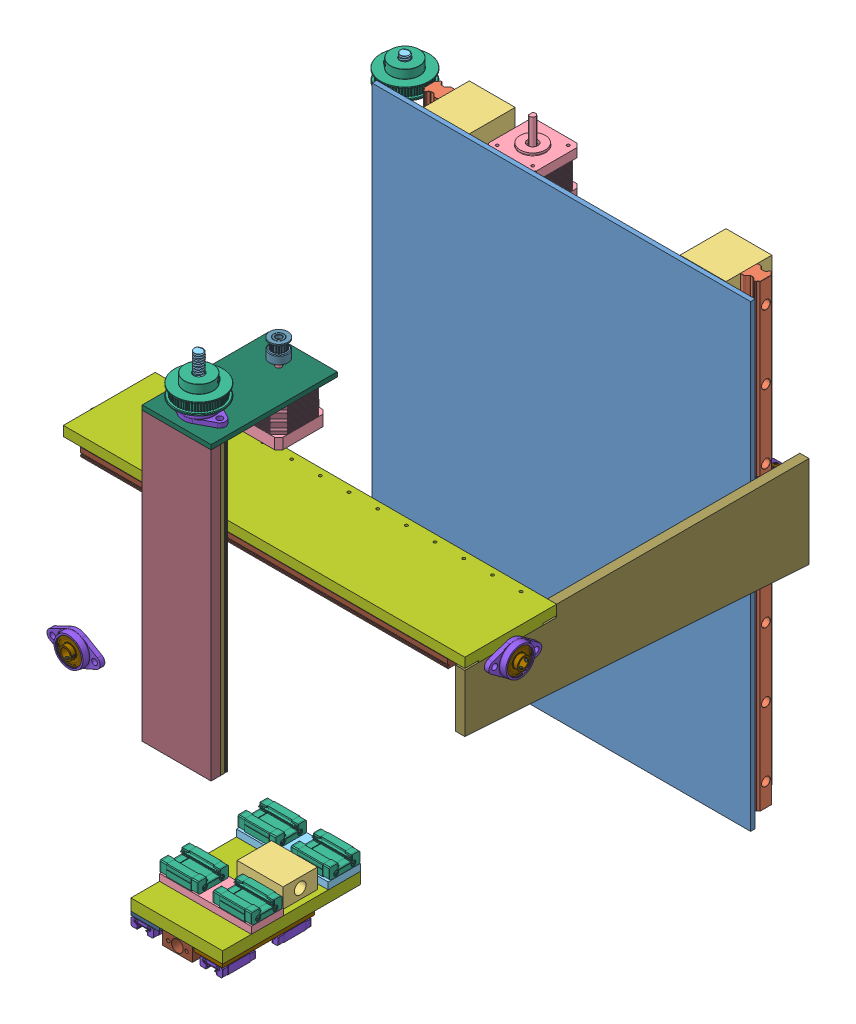
SolidWorks assembly Fresa_190421_2259, configuration Predeterminado. Lengths in mm.
Overall size (378.35 507.31 471.29).
73 component instances, 35 part files, 0 mates.
Components (placement in the parent):
- Mesa^Fresa_190421_2259-1: Mesa^Fresa_190421_2259 [Predeterminado] at (-186.1122 103.6393 -218.5133) x (0 -1 0) z (0 0 1) size (400 330 4) (virtual)
- HGR15R Rail-1: HGR15R Rail [HGR15R400CE20] at (-145.2122 -296.3607 -238.5133) x (0 0 1) z (0 -1 0) size (15 15 400)
- perfil_4040^Fresa_190421_2259-1: perfil_4040^Fresa_190421_2259 [Predeterminado] at (-145.3622 103.6393 -258.5133) x (1 0 0) z (0 -1 0) size (40 40 400) (virtual)
- HGR15R Rail-2: HGR15R Rail [HGR15R400CE20] at (117.8878 -296.3607 -238.8633) x (0 0 -1) z (0 -1 0) size (15 15 400)
- perfil_4040^Fresa_190421_2259-2: perfil_4040^Fresa_190421_2259 [Predeterminado] at (78.0378 103.6393 -258.8633) x (1 0 0) z (0 -1 0) size (40 40 400) (virtual)
- Nema 17HS4401-S-2: Nema 17HS4401-S [Varsayılan] at (-71.0952 61.4393 -239.5133) x (0 0 -1) z (0 1 0) size (42 48 63.23)
- LeadScrew 8mm x 2mmPitch-2: LeadScrew 8mm x 2mmPitch [Default] at (-180.6122 117.9173 -237.6496) x (0.520198 0 -0.854046) z (0 1 0) size (9.24 8 301.1)
- GT2_60T_8_6-2: GT2_60T_8_6 [Default] at (-180.6122 106.533 -237.6496) x (-0.750477 0 -0.660897) z (0 -1 0) size (42 42 18)
- Eje_X^Fresa_190421_2259-1: Eje_X^Fresa_190421_2259 [Predeterminado] at (0 -20.7118 0) size (378.35 85.52 428.57) (virtual)
  - Copia de Placa_X^Eje_X_Fresa_190421_2259-1: Copia de Placa_X^Eje_X_Fresa_190421_2259 [Predeterminado] at (-196.1122 -9.5232 -35.4133) x (1 0 0) z (0 -1 0) size (350 80 10) (virtual)
  - KFL08-1: KFL08 [Varsayılan] at (-66.4126 -53.0232 161.3598) x (0.999067 -0.043192 0) z (-0.043192 -0.999067 0) size (46.5 11.35 27)
    - FLANGE^KFL08-1: FLANGE^KFL08 [Default] at origin size (46.5 8.5 27) (virtual)
    - BEARING^KFL08-1: BEARING^KFL08 [Default] at (0 4 0) x (1 0 0) z (0 -1 0) size (22 22 10.85) (virtual)
    - socket set screw cone point_am-1: socket set screw cone point_am [B18.3.6M - M2.5 x 0.45 x 2 Hex Socket Cone Pt. SS --S] at (0 9.425 5.45) x (0 0 -1) z (1 0 0) size (2 2.5 2.5)
    - socket set screw cone point_am-2: socket set screw cone point_am [B18.3.6M - M2.5 x 0.45 x 2 Hex Socket Cone Pt. SS --S] at (5.45 9.425 0) x (-1 0 0) z (0 0 -1) size (2 2.5 2.5)
  - LeadScrew 8mm x 2mmPitch-1: LeadScrew 8mm x 2mmPitch [Default] at (-212.2662 -28.5232 4.5867) x (0 0.930056 0.367419) z (-1 0 0) size (9.24 8 301.1)
  - MGN12R-320-1: MGN12R-320 [Predeterminado] at (-111.1122 -21.9725 -29.4133) x (0 0 1) z (1 0 0) size (12 8.1 320)
  - MGN12R-320-2: MGN12R-320 [Predeterminado] at (-111.1122 -21.9725 38.5867) x (0 0 1) z (1 0 0) size (12 8.1 320)
  - Copia de Columa_1^Eje_X_Fresa_190421_2259-1: Copia de Columa_1^Eje_X_Fresa_190421_2259 [Predeterminado] at (-188.1122 -29.0154 -199.7436) x (0 -1 0) z (-1 0 0) size (80 300 8) (hidden, virtual)
  - Copia de Columa_1^Eje_X_Fresa_190421_2259-2: Copia de Columa_1^Eje_X_Fresa_190421_2259 [Predeterminado] at (153.8878 -29.0154 -199.7436) x (0 -1 0) z (-1 0 0) size (80 300 8) (virtual)
  - HGH15CA-1: HGH15CA [Default] at (117.8878 -53.7232 -238.8633) x (0 0 -1) z (0 -1 0) size (34 23.7 61.49)
    - HGH15CA Block-1: HGH15CA Block [HGR15R300CE20] at origin size (34 23.7 39.4)
    - HGx15CA Retainer-1: HGx15CA Retainer [HGR15R300CE20] at origin size (26 4 55.4)
    - HGx15CA Tiny Red-1: HGx15CA Tiny Red [HGR15R300CE20] at origin size (14.2 1 55.4)
    - HGx15CA End Cap-1: HGx15CA End Cap [HGR15R300CE20] at origin size (32.5 19.5 8)
    - HGx15CA End Cap-2: HGx15CA End Cap [HGR15R300CE20] x (-1 0 0) z (0 0 -1) size (32.5 19.5 8)
    - HGx15CA Seal-1: HGx15CA Seal [HGR15R300CE20] at origin size (32.5 19.5 3)
    - HGx15CA Seal-2: HGx15CA Seal [HGR15R300CE20] x (-1 0 0) z (0 0 -1) size (32.5 19.5 3)
    - pan head cross recess screw_iso2-1: pan head cross recess screw_iso2 [ISO 7045 - M2.5 x 16 - Z - 16C] at (11.5 11.8 30.8) x (0 0 -1) z (0 -1 0) size (18.05 5 5)
    - pan head cross recess screw_iso2-2: pan head cross recess screw_iso2 [ISO 7045 - M2.5 x 16 - Z - 16C] at (-11.5 11.8 30.8) x (0 0 -1) z (0 1 0) size (18.05 5 5)
    - pan head cross recess screw_iso2-3: pan head cross recess screw_iso2 [ISO 7045 - M2.5 x 16 - Z - 16C] at (11.5 11.8 -30.8) x (0 0 1) z (0 -1 0) size (18.05 5 5)
    - pan head cross recess screw_iso2-4: pan head cross recess screw_iso2 [ISO 7045 - M2.5 x 16 - Z - 16C] at (-11.5 11.8 -30.8) x (0 0 1) z (0 1 0) size (18.05 5 5)
  - Copia de Soporte_tuerca_husillo_X^Eje_X_Fresa_190421_2259-1: Copia de Soporte_tuerca_husillo_X^Eje_X_Fresa_190421_2259 [Predeterminado] at (-188.1122 -9.5232 -219.4133) x (0 -1 0) z (1 0 0) size (60 36 15) (virtual)
  - KFL08-2: KFL08 [Varsayılan] at (153.8878 -28.5232 4.5867) x (0 -0.14239 -0.989811) z (0 -0.989811 0.14239) size (46.5 11.35 27)
    - FLANGE^KFL08-1: FLANGE^KFL08 [Default] at origin size (46.5 8.5 27) (virtual)
    - BEARING^KFL08-1: BEARING^KFL08 [Default] at (0 4 0) x (1 0 0) z (0 -1 0) size (22 22 10.85) (virtual)
    - socket set screw cone point_am-1: socket set screw cone point_am [B18.3.6M - M2.5 x 0.45 x 2 Hex Socket Cone Pt. SS --S] at (0 9.425 5.45) x (0 0 -1) z (1 0 0) size (2 2.5 2.5)
    - socket set screw cone point_am-2: socket set screw cone point_am [B18.3.6M - M2.5 x 0.45 x 2 Hex Socket Cone Pt. SS --S] at (5.45 9.425 0) x (-1 0 0) z (0 0 -1) size (2 2.5 2.5)
  - LeadScrew Nut 8mm x 2mmPitch-1: LeadScrew Nut 8mm x 2mmPitch [Default] at (-180.6122 -6.0232 -237.6496) x (-0.798509 0 -0.601983) z (0 1 0) size (22 22 16.05)
- Eje_Y^Fresa_190421_2259-1: Eje_Y^Fresa_190421_2259 [Predeterminado] at (122.2851 -161.5666 169.038) size (81.36 44.81 120.46) (virtual)
  - Copia de Alojamiento_tuerca_Y^Eje_Y_Fresa_190421_2259-1: Copia de Alojamiento_tuerca_Y^Eje_Y_Fresa_190421_2259 [Predeterminado] at (-25.6004 -20.0232 -23.0978) x (-1 0 0) z (0 -1 0) size (40 30 17) (virtual)
  - Copia de Alza_patines_A^Eje_Y_Fresa_190421_2259-1: Copia de Alza_patines_A^Eje_Y_Fresa_190421_2259 [Predeterminado] at (-100.6004 -31.0232 -18.5043) x (1 0 0) z (0 -1 0) size (80 28 6) (virtual)
  - Copia de Alza_patines_B^Eje_Y_Fresa_190421_2259-1: Copia de Alza_patines_B^Eje_Y_Fresa_190421_2259 [Predeterminado] at (-100.6004 -31.0232 -85.5043) x (1 0 0) z (0 -1 0) size (80 28 6) (virtual)
  - MGN12C-1: MGN12C [Default] at (-28.259 -21.0071 -68.6923) x (0 0 -1) z (-1 0 0) size (27 10 34.86)
  - MGN12C-2: MGN12C [Default] at (-74.759 -21.0071 -68.6923) x (0 0 -1) z (-1 0 0) size (27 10 34.86)
  - MGN12C-3: MGN12C [Default] at (-74.759 -21.0071 -0.6923) x (0 0 -1) z (-1 0 0) size (27 10 34.86)
  - MGN12C-4: MGN12C [Default] at (-28.259 -21.0071 -0.6923) x (0 0 -1) z (-1 0 0) size (27 10 34.86)
  - Copia de Placa_Z^Eje_Y_Fresa_190421_2259-1: Copia de Placa_Z^Eje_Y_Fresa_190421_2259 [Predeterminado] at (-100.6004 -37.0232 -85.5043) x (1 0 0) z (0 -1 0) size (80 120 10) (virtual)
  - MGN9C-1: MGN9C [Default] at (-27.8201 -54.6723 19.1196) size (20 8 29.63)
  - MGN9C-2: MGN9C [Default] at (-87.8201 -54.6723 19.1196) size (20 8 29.63)
  - MGN9C-3: MGN9C [Default] at (-87.8201 -54.6723 -29.5804) size (20 8 29.63)
  - MGN9C-4: MGN9C [Default] at (-27.8201 -54.6723 -29.5804) size (20 8 29.63)
  - Copia de Alza_eje_Z_A^Eje_Y_Fresa_190421_2259-1: Copia de Alza_eje_Z_A^Eje_Y_Fresa_190421_2259 [Predeterminado] at (-20.6004 -50.0232 -45.5043) x (-1 0 0) z (0 1 0) size (25 80 3) (virtual)
  - Copia de Alza_eje_Z_B^Eje_Y_Fresa_190421_2259-1: Copia de Alza_eje_Z_B^Eje_Y_Fresa_190421_2259 [Predeterminado] at (-75.6004 -50.0232 -45.5043) x (-1 0 0) z (0 1 0) size (25 80 3) (virtual)
  - Copia de Alojamiento_tuerca_ejeZ^Eje_Y_Fresa_190421_2259-1: Copia de Alojamiento_tuerca_ejeZ^Eje_Y_Fresa_190421_2259 [Predeterminado] at (-47.0572 -47.0232 14.4957) x (-1 0 0) z (0 0 1) size (26 12 20) (virtual)
  - LeadScrew Nut 8mm x 2mmPitch-1: LeadScrew Nut 8mm x 2mmPitch [Default] at (-66.4126 -53.0232 -46.4043) x (-0.997082 -0.076335 0) z (0 0 -1) size (22 22 16.05)
- Eje_Z^Fresa_190421_2259-1: Eje_Z^Fresa_190421_2259 [Predeterminado] at (6.3905 15.2486 43.2497) size (60 301.1 125.53) (virtual)
  - MGN9R-250-1: MGN9R-250 [Predeterminado] at (15.2598 -105.1519 134.6514) x (1 0 0) z (0 1 0) size (9 6.61 250)
  - Copia de Placa_Motor^Eje_Z_Fresa_190421_2259-1: Copia de Placa_Motor^Eje_Z_Fresa_190421_2259 [Predeterminado] at (70.7598 -105.1519 145.8457) x (-1 0 0) z (0 0 -1) size (60 250 8) (virtual)
  - MGN9R-250-2: MGN9R-250 [Predeterminado] at (66.2598 -105.1519 134.6514) x (1 0 0) z (0 1 0) size (9 6.61 250)
  - Nema 17HS4401-S-1: Nema 17HS4401-S [Varsayılan] at (40.7598 104.6481 56.8457) x (1 0 0) z (0 1 0) size (42 48 63.23)
  - GT2_60T_8_6-1: GT2_60T_8_6 [Default] at (40.3385 170.6578 126.1426) x (0.820472 0 -0.571687) z (0 -1 0) size (42 42 18)
  - GT2_20T-1: GT2_20T [Конфигурация1] at (40.7598 154.7078 56.8457) x (0 1 0) z (-0.802397 0 -0.596791) size (16 16 16)
  - Copia de soporte_motor_Z^Eje_Z_Fresa_190421_2259-1: Copia de soporte_motor_Z^Eje_Z_Fresa_190421_2259 [Predeterminado] at (10.7598 148.8481 145.8457) x (0 0 -1) z (0 -1 0) size (110 60 4) (virtual)
  - LeadScrew 8mm x 2mmPitch-1: LeadScrew 8mm x 2mmPitch [Default] at (40.3385 194.8481 126.1426) x (0.619003 0 -0.785388) z (0 1 0) size (9.24 8 301.1)
  - KFL08-1: KFL08 [Varsayılan] at (40.3385 148.8481 126.1426) size (46.5 11.35 27)
    - FLANGE^KFL08-1: FLANGE^KFL08 [Default] at origin size (46.5 8.5 27) (virtual)
    - BEARING^KFL08-1: BEARING^KFL08 [Default] at (0 4 0) x (1 0 0) z (0 -1 0) size (22 22 10.85) (virtual)
    - socket set screw cone point_am-1: socket set screw cone point_am [B18.3.6M - M2.5 x 0.45 x 2 Hex Socket Cone Pt. SS --S] at (0 9.425 5.45) x (0 0 -1) z (1 0 0) size (2 2.5 2.5)
    - socket set screw cone point_am-2: socket set screw cone point_am [B18.3.6M - M2.5 x 0.45 x 2 Hex Socket Cone Pt. SS --S] at (5.45 9.425 0) x (-1 0 0) z (0 0 -1) size (2 2.5 2.5)
- Cabezal^Fresa_190421_2259-1: Cabezal^Fresa_190421_2259 [Predeterminado] at (-4.1094 3.4062 -13.81) size (42 42 75) (hidden, virtual)
  - Cuerpo^Cabezal_Fresa_190421_2259-1: Cuerpo^Cabezal_Fresa_190421_2259 [Predeterminado] at origin size (42 42 74) (virtual)
  - Sup^Cabezal_Fresa_190421_2259-1: Sup^Cabezal_Fresa_190421_2259 [Predeterminado] at origin size (42 42 6) (virtual)
